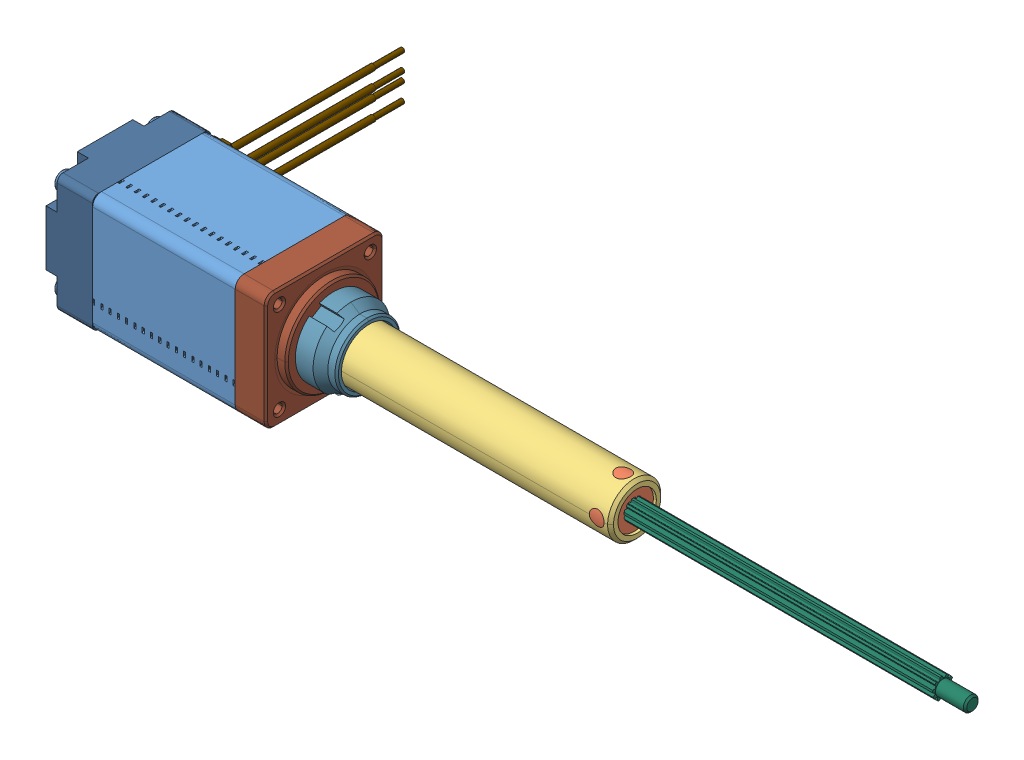
SolidWorks assembly 20K-2M..50, configuration 默认. Lengths in mm.
Overall size (146.95 25.88 47.14).
32 component instances, 21 part files, 0 mates.
Components (placement in the parent):
- 20K-2M..50.STEP-1: 20K-2M..50.STEP [默认] at origin size (146.95 25.88 47.14)
  - 02-20-42.STEP-1: 02-20-42.STEP [默认] at (19.975 0 0) x (0 -1 0) z (-1 0 0) size (25.88 26.04 31.85)
    - 02-20-24.15_10-20-001-2.STEP-1: 02-20-24.15_10-20-001-2.STEP [默认] at origin size (20 20 24.15)
    - 13-20-12.5____.STEP-1: 13-20-12.5____.STEP [默认] at (0 0 16.075) x (-1 0 0) z (0 0 -1) size (18.2 22.2 16.51)
    - 13-20-12.5______.STEP-1: 13-20-12.5______.STEP [默认] at (0 0 -14.575) x (0.707107 0.707107 0) z (0 0 1) size (18.3 18.3 15.8)
    - 20-20__________.STEP-1: 20-20__________.STEP [默认] at (0 0 15.675) size (17.8 21 0.9)
    - 13-20-001________.STEP-1: 13-20-001________.STEP [默认] at (0 -8.6 12.175) x (1 0 0) z (0 0 -1) size (10.5 7.2 3.5)
  - 03-20-006____42_____default.STEP-1: 03-20-006____42_____default.STEP [默认] at (5.7 0 0) x (1 0 0) z (0 0.381126 -0.924523) size (29.65 16.26 16.27)
    - 06-20-006____42______YK_01-20-007-1.STEP-1: 06-20-006____42______YK_01-20-007-1.STEP [默认] at origin size (29.65 7 7)
    - 03-20-4.2-6YK_10-20-006-2.STEP-1: 03-20-4.2-6YK_10-20-006-2.STEP [默认] at (22.53 0 0) x (0 0.91534 0.402682) z (-1 0 0) size (12.06 12.08 4.24)
    - 10-20-001__________.STEP-1: 10-20-001__________.STEP [默认] at (14.67 0 0) x (0 0 1) z (-1 0 0) size (11 11 1)
    - 08-20-001_____07-20-001-1.STEP-1: 08-20-001_____07-20-001-1.STEP [默认] at (20.41 0 0) x (0 0 1) z (-1 0 0) size (11 11 1.5)
    - 08-20-001_____07-20-001-1.STEP-2: 08-20-001_____07-20-001-1.STEP [默认] at (9.43 0 0) x (0 0 1) z (-1 0 0) size (11 11 1.5)
    - 03-20-4.2-6YK_10-20-006-2.STEP-2: 03-20-4.2-6YK_10-20-006-2.STEP [默认] at (16.79 0 0) x (0 0.888249 0.459362) z (-1 0 0) size (12.06 12.08 4.24)
    - 03-20-4.2-6YK_10-20-006-2.STEP-3: 03-20-4.2-6YK_10-20-006-2.STEP [默认] at (11.55 0 0) x (0 0.91534 0.402682) z (-1 0 0) size (12.06 12.08 4.24)
    - 03-20-4.2-6YK_10-20-006-2.STEP-4: 03-20-4.2-6YK_10-20-006-2.STEP [默认] at (5.81 0 0) x (0 0.888249 0.459362) z (-1 0 0) size (12.06 12.08 4.24)
  - 01-20-006__20__________YK__.STEP-1: 01-20-006__20__________YK__.STEP [默认] at origin size (8.8 20 20)
  - 01-20-005(20____________YK__.STEP-1: 01-20-005(20____________YK__.STEP [默认] at (31.25 0 0) x (0 0 -1) z (1 0 0) size (20 20 7.5)
  - 09-20-001____9X__5X4)_09-20-001.STEP-1: 09-20-001____9X__5X4)_09-20-001.STEP [默认] at (5.7 0 0) x (1 0 0) z (0 0.998527 -0.054257) size (3 9 9)
  - 09-20-001____9X__5X4)_09-20-001.STEP-2: 09-20-001____9X__5X4)_09-20-001.STEP [默认] at (32.35 0 0) x (1 0 0) z (0 0.945037 0.326964) size (3 9 9)
  - 06-20-017__20________YK___20____________YK.STEP-1: 06-20-017__20________YK___20____________YK.STEP [默认] at (30.35 0 0) x (0 0.924523 0.381126) z (-1 0 0) size (6.01 6.01 10)
  - 07-20-007__________________.STEP-1: 07-20-007__________________.STEP [默认] at (38.75 0 0) x (-1 0 0) z (0 -0.999857 -0.016895) size (6 12.92 13)
  - 07-20-015-1______________.STEP-1: 07-20-015-1______________.STEP [默认] at (82.15 0 0) x (0 -0.714016 0.700129) z (1 0 0) size (3.42 3.5 64.8)
  - 07-20-015-2______________.STEP-1: 07-20-015-2______________.STEP [默认] at (20.35 0 0) x (0 0.924225 0.381849) z (1 0 0) size (3.5 3.9 64.81)
  - 07-20-006__20______.STEP-1: 07-20-006__20______.STEP [默认] at (86.15 0 0) x (0 0.924225 0.381849) z (1 0 0) size (3.9 4.45 0.4)
  - 14-20-001__20-28____________________.STEP-1: 14-20-001__20-28____________________.STEP [默认] at (6.48 -0.2 -10) x (0 -1 0) z (0 0 1) size (10.5 3.4 24.5)
  - 11-20-001__M2-24.5__20-30__.STEP-1: 11-20-001__M2-24.5__20-30__.STEP [默认] at (0.39 7.7 -7.7) x (0 -0.010787 -0.999942) z (1 0 0) size (3 3 26)
  - 11-20-001__M2-24.5__20-30__.STEP-2: 11-20-001__M2-24.5__20-30__.STEP [默认] at (0.39 7.7 7.7) x (0 0.999942 -0.010787) z (1 0 0) size (3 3 26)
  - 11-20-001__M2-24.5__20-30__.STEP-3: 11-20-001__M2-24.5__20-30__.STEP [默认] at (0.39 -7.7 7.7) x (0 0.010787 0.999942) z (1 0 0) size (3 3 26)
  - 11-20-001__M2-24.5__20-30__.STEP-4: 11-20-001__M2-24.5__20-30__.STEP [默认] at (0.39 -7.7 -7.7) x (0 -0.999942 0.010787) z (1 0 0) size (3 3 26)
  - 07-20-002__20________________.STEP-1: 07-20-002__20________________.STEP [默认] at (87.8 0 0) x (0 0 -1) z (1 0 0) size (9.01 9.01 3.1)
  - 07-20-015-3__20_____________08-20-002-1.STEP-1: 07-20-015-3__20_____________08-20-002-1.STEP [默认] at (35.35 0 0) x (0 0 -1) z (1 0 0) size (9.01 9.01 54.8)
